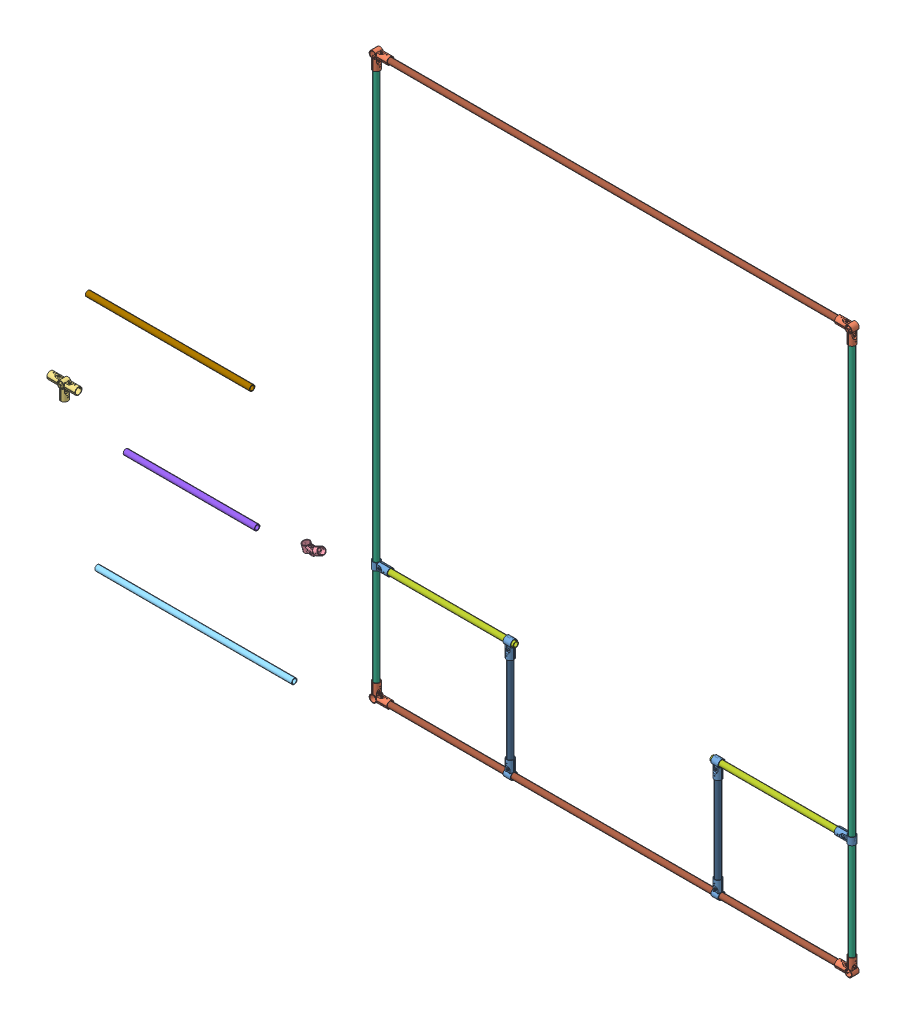
SolidWorks assembly SteelTubeAssembly, configuration Default. Lengths in mm.
Overall size (3905.99 2753.98 797.75).
23 component instances, 11 part files, 50 mates.
Components (placement in the parent):
- 2534T210_CLAMP-ON FRAMING FITTING-2: 2534T210_CLAMP-ON FRAMING FITTING [2534T21] at (584.2 0 0) x (1 0 0) z (0 0 -1) size (33.53 82.55 34.1)
- 2534T240_CLAMP-ON FRAMING FITTING-1: 2534T240_CLAMP-ON FRAMING FITTING [2534T24] at (2171.7 0 0) x (-1 0 0) z (0 0 1) size (81.85 81.28 33.46)
- 2534T260_CLAMP-ON FRAMING FITTING-1: 2534T260_CLAMP-ON FRAMING FITTING [2534T26] at (-1430.376 594.6399 57.1912) size (130.05 82.36 33.46)
- 2534T330_CLAMP-ON FRAMING FITTING-1: 2534T330_CLAMP-ON FRAMING FITTING [2534T33] at (46.223 849.693 406.2699) x (0.990082 0.041139 0.134332) z (-0.122317 -0.217936 0.968268) size (113.89 62.11 35.25)
- Depth Bar-1: Depth Bar [Default] at (-1338.4664 -133.7185 -4.7662) size (914.4 25.4 25.4)
- Height-1: Height [Default] at (2171.7 2552.7 0) x (0 -1 0) z (-0.85323 0 -0.521535) size (2514.6 25.4 25.4)
- Horizonal Corner-1: Horizonal Corner [Default] at (0 533.4 0) size (609.6 25.4 25.4)
- Lower Mounting Bar-1: Lower Mounting Bar [Default] at (-1489.6692 115.3649 -288.1125) size (609.6 25.4 25.4)
- Upper Mounting Bar-1: Upper Mounting Bar [Default] at (-1716.8304 613.4329 -339.6472) size (762 25.4 25.4)
- Vertical Corner-1: Vertical Corner [Default] at (584.2 495.3 0) x (0 -1 0) z (-0.899193 0 0.437553) size (457.2 25.4 25.4)
- Width-1: Width [Default] at origin size (2133.6 25.4 25.4)
- 2534T240_CLAMP-ON FRAMING FITTING-2: 2534T240_CLAMP-ON FRAMING FITTING [2534T24] at (2171.7 2590.8 0) x (-1 0 0) z (0 0 -1) size (81.85 81.28 33.46)
- 2534T240_CLAMP-ON FRAMING FITTING-5: 2534T240_CLAMP-ON FRAMING FITTING [2534T24] at (-38.1 0 0) x (1 0 0) z (0 0 -1) size (81.85 81.28 33.46)
- Height-3: Height [Default] at (-38.1 2552.7 0) x (0 -1 0) z (-0.845396 0 -0.534139) size (2514.6 25.4 25.4)
- 2534T240_CLAMP-ON FRAMING FITTING-6: 2534T240_CLAMP-ON FRAMING FITTING [2534T24] at (-38.1 2590.8 0) size (81.85 81.28 33.46)
- Width-3: Width [Default] at (0 2590.8 0) x (1 0 0) z (0 0.262637 0.964895) size (2133.6 25.4 25.4)
- 2534T210_CLAMP-ON FRAMING FITTING-3: 2534T210_CLAMP-ON FRAMING FITTING [2534T21] at (584.2 533.4 0) size (33.53 82.55 34.1)
- 2534T210_CLAMP-ON FRAMING FITTING-5: 2534T210_CLAMP-ON FRAMING FITTING [2534T21] at (-38.1 533.4 0) x (0 -1 0) z (0 0 -1) size (33.53 82.55 34.1)
- 2534T210_CLAMP-ON FRAMING FITTING-10: 2534T210_CLAMP-ON FRAMING FITTING [2534T21] at (1549.4 0 0) x (1 0 0) z (0 0 -1) size (33.53 82.55 34.1)
- 2534T210_CLAMP-ON FRAMING FITTING-11: 2534T210_CLAMP-ON FRAMING FITTING [2534T21] at (1549.4 533.4 0) x (-1 0 0) z (0 0 -1) size (33.53 82.55 34.1)
- Vertical Corner-3: Vertical Corner [Default] at (1549.4 495.3 0) x (0 -1 0) z (-0.962184 0 -0.272399) size (457.2 25.4 25.4)
- Horizonal Corner-3: Horizonal Corner [Default] at (1524 533.4 0) x (1 0 0) z (0 -0.195703 0.980663) size (609.6 25.4 25.4)
- 2534T210_CLAMP-ON FRAMING FITTING-12: 2534T210_CLAMP-ON FRAMING FITTING [2534T21] at (2171.7 533.4 0) x (0 -1 0) z (0 0 1) size (33.53 82.55 34.1)
Mates (geometry in assembly coordinates):
- Coincident1: coordinate: point of Width-1; point of assembly
- Concentric1: concentric anti-aligned: cylinder of 2534T240_CLAMP-ON FRAMING FITTING-1 through (2107.184 0 0) axis (1 0 0) radius 13.97; cylinder of Width-1 through (2133.6 0 0) axis (-1 0 0) radius 12.7
- Distance1: distance = 38.1 mm: point of 2534T240_CLAMP-ON FRAMING FITTING-1; plane of Width-1 through (2133.6 0 0) normal (1 0 0)
- Coincident2: coincident aligned: plane of Width-1 through (0 0 0) normal (0 0 1); plane of assembly through (0 0 0) normal (0 0 1)
- Parallel1: parallel aligned: plane of 2534T240_CLAMP-ON FRAMING FITTING-1 through (2171.7 64.516 0) normal (0 1 0); plane of assembly through (0 0 0) normal (0 1 0)
- Concentric2: concentric anti-aligned: cylinder of 2534T240_CLAMP-ON FRAMING FITTING-1 through (2171.7 64.516 0) axis (0 -1 0) radius 13.97; cylinder of Height-1 through (2171.7 38.1 0) axis (0 1 0) radius 12.7
- Distance2: distance = 38.1 mm anti-aligned: plane of Height-1 through (2171.7 38.1 0) normal (0 -1 0); plane of Width-1 through (0 0 0) normal (0 1 0)
- Concentric3: concentric aligned: cylinder of Height-1 through (2171.7 38.1 0) axis (0 1 0) radius 12.7; cylinder of 2534T240_CLAMP-ON FRAMING FITTING-2 through (2171.7 2526.284 0) axis (0 1 0) radius 13.97
- Distance3: distance = 38.1 mm: plane of Height-1 through (2171.7 2552.7 0) normal (0 1 0); point of 2534T240_CLAMP-ON FRAMING FITTING-2
- Parallel2: parallel aligned: plane of 2534T240_CLAMP-ON FRAMING FITTING-2 through (2171.7 2590.8 16.73) normal (0 0 1); plane of assembly through (0 0 0) normal (0 0 1)
- Concentric13: concentric aligned: cylinder of Width-1 through (2133.6 0 0) axis (-1 0 0) radius 12.7; cylinder of 2534T240_CLAMP-ON FRAMING FITTING-5 through (26.416 0 0) axis (-1 0 0) radius 13.97
- Distance9: distance = 38.1 mm: plane of Width-1 through (0 0 0) normal (-1 0 0); point of 2534T240_CLAMP-ON FRAMING FITTING-5
- Parallel5: parallel aligned: plane of 2534T240_CLAMP-ON FRAMING FITTING-1 through (2171.7 64.516 0) normal (0 1 0); plane of 2534T240_CLAMP-ON FRAMING FITTING-5 through (-38.1 64.516 0) normal (0 1 0)
- Concentric14: concentric anti-aligned: cylinder of 2534T240_CLAMP-ON FRAMING FITTING-5 through (-38.1 64.516 0) axis (0 -1 0) radius 13.97; cylinder of Height-3 through (-38.1 38.1 0) axis (0 1 0) radius 12.7
- Distance10: distance = 38.1 mm: plane of Height-3 through (-38.1 38.1 0) normal (0 -1 0); point of 2534T240_CLAMP-ON FRAMING FITTING-5
- Concentric15: concentric aligned: cylinder of Height-3 through (-38.1 38.1 0) axis (0 1 0) radius 12.7; cylinder of 2534T240_CLAMP-ON FRAMING FITTING-6 through (-38.1 2526.284 0) axis (0 1 0) radius 13.97
- Distance11: distance = 38.1 mm: plane of Height-3 through (-38.1 2552.7 0) normal (0 1 0); point of 2534T240_CLAMP-ON FRAMING FITTING-6
- Parallel6: parallel aligned: plane of Height-1 through (2171.7 2552.7 0) normal (0 1 0); plane of Height-3 through (-38.1 2552.7 0) normal (0 1 0)
- Concentric16: concentric anti-aligned: cylinder of 2534T240_CLAMP-ON FRAMING FITTING-2 through (2107.184 2590.8 0) axis (1 0 0) radius 13.97; cylinder of Width-3 through (2133.6 2590.8 0) axis (-1 0 0) radius 12.7
- Distance12: distance = 38.1 mm: point of 2534T240_CLAMP-ON FRAMING FITTING-2; plane of Width-3 through (2133.6 2590.8 0) normal (1 0 0)
- Parallel8: parallel anti-aligned: plane of 2534T240_CLAMP-ON FRAMING FITTING-2 through (2107.184 2590.8 0) normal (-1 0 0); plane of 2534T240_CLAMP-ON FRAMING FITTING-6 through (26.416 2590.8 0) normal (1 0 0)
- Concentric19: concentric aligned: cylinder of 2534T210_CLAMP-ON FRAMING FITTING-2 through (600.964 0 0) axis (-1 0 0) radius 13.97; cylinder of Width-1 through (2133.6 0 0) axis (-1 0 0) radius 12.7
- Parallel9: parallel aligned: plane of 2534T210_CLAMP-ON FRAMING FITTING-2 through (584.2 65.786 0) normal (0 1 0); plane of 2534T240_CLAMP-ON FRAMING FITTING-5 through (-38.1 64.516 0) normal (0 1 0)
- Concentric20: concentric anti-aligned: cylinder of 2534T210_CLAMP-ON FRAMING FITTING-2 through (584.2 65.786 0) axis (0 -1 0) radius 13.97; cylinder of Vertical Corner-1 through (584.2 38.1 0) axis (0 1 0) radius 12.7
- Distance13: distance = 38.1 mm: point of 2534T210_CLAMP-ON FRAMING FITTING-2; plane of Vertical Corner-1 through (584.2 38.1 0) normal (0 -1 0)
- Concentric24: concentric aligned: cylinder of Vertical Corner-1 through (584.2 38.1 0) axis (0 1 0) radius 12.7; cylinder of 2534T210_CLAMP-ON FRAMING FITTING-3 through (584.2 467.614 0) axis (0 1 0) radius 13.97
- Distance14: distance = 38.1 mm: point of 2534T210_CLAMP-ON FRAMING FITTING-3; plane of Vertical Corner-1 through (584.2 495.3 0) normal (0 1 0)
- Concentric25: concentric anti-aligned: cylinder of Height-3 through (-38.1 38.1 0) axis (0 1 0) radius 12.7; cylinder of 2534T210_CLAMP-ON FRAMING FITTING-5 through (-38.1 550.164 0) axis (0 -1 0) radius 13.97
- Parallel10: parallel aligned: plane of 2534T240_CLAMP-ON FRAMING FITTING-5 through (26.416 0 0) normal (1 0 0); plane of 2534T210_CLAMP-ON FRAMING FITTING-5 through (27.686 533.4 0) normal (1 0 0)
- Parallel11: parallel anti-aligned: plane of 2534T210_CLAMP-ON FRAMING FITTING-3 through (567.436 533.4 0) normal (-1 0 0); plane of 2534T210_CLAMP-ON FRAMING FITTING-5 through (27.686 533.4 0) normal (1 0 0)
- Concentric26: concentric aligned: cylinder of Horizonal Corner-1 through (609.6 533.4 0) axis (-1 0 0) radius 12.7; cylinder of 2534T210_CLAMP-ON FRAMING FITTING-3 through (600.964 533.4 0) axis (-1 0 0) radius 13.97
- Distance15: distance = 25.4 mm: point of 2534T210_CLAMP-ON FRAMING FITTING-3; plane of Horizonal Corner-1 through (609.6 533.4 0) normal (1 0 0)
- Distance16: distance = 38.1 mm: plane of Horizonal Corner-1 through (0 533.4 0) normal (-1 0 0); point of 2534T210_CLAMP-ON FRAMING FITTING-5
- Concentric27: concentric aligned: cylinder of Horizonal Corner-1 through (609.6 533.4 0) axis (-1 0 0) radius 12.7; cylinder of 2534T210_CLAMP-ON FRAMING FITTING-5 through (27.686 533.4 0) axis (-1 0 0) radius 13.97
- Concentric28: concentric aligned: cylinder of ? through (569.8292 2128.6091 5503.5233) axis (0 1 0) radius 12.7; cylinder of ? through (569.8292 2558.1231 5503.5233) axis (0 1 0) radius 13.97
- Distance17: distance = 25.4 mm: point of ?; plane of ? through (595.2292 2623.9091 5503.5233) normal (1 0 0)
- Distance19: distance = 38.1 mm: point of ?; plane of ? through (569.8292 2585.8091 5503.5233) normal (0 1 0)
- Concentric30: concentric aligned: cylinder of ? through (595.2292 2623.9091 5503.5233) axis (-1 0 0) radius 12.7; cylinder of ? through (586.5932 2623.9091 5503.5233) axis (-1 0 0) radius 13.97
- Concentric31: concentric anti-aligned: cylinder of Width-1 through (2133.6 0 0) axis (-1 0 0) radius 12.7; cylinder of 2534T210_CLAMP-ON FRAMING FITTING-10 through (1532.636 0 0) axis (1 0 0) radius 13.97
- Concentric32: concentric anti-aligned: cylinder of 2534T210_CLAMP-ON FRAMING FITTING-10 through (1549.4 65.786 0) axis (0 -1 0) radius 13.97; cylinder of Vertical Corner-3 through (1549.4 38.1 0) axis (0 1 0) radius 12.7
- Distance20: distance = 38.1 mm: plane of Vertical Corner-3 through (1549.4 38.1 0) normal (0 -1 0); point of 2534T210_CLAMP-ON FRAMING FITTING-10
- Concentric33: concentric aligned: cylinder of 2534T210_CLAMP-ON FRAMING FITTING-11 through (1549.4 467.614 0) axis (0 1 0) radius 13.97; cylinder of Vertical Corner-3 through (1549.4 38.1 0) axis (0 1 0) radius 12.7
- Parallel12: parallel aligned: plane of 2534T240_CLAMP-ON FRAMING FITTING-1 through (2171.7 64.516 0) normal (0 1 0); plane of Vertical Corner-3 through (1549.4 495.3 0) normal (0 1 0)
- Distance21: distance = 38.1 mm: point of 2534T210_CLAMP-ON FRAMING FITTING-11; plane of Vertical Corner-3 through (1549.4 495.3 0) normal (0 1 0)
- Parallel13: parallel anti-aligned: plane of 2534T210_CLAMP-ON FRAMING FITTING-3 through (600.964 533.4 0) normal (1 0 0); plane of 2534T210_CLAMP-ON FRAMING FITTING-11 through (1532.636 533.4 0) normal (-1 0 0)
- Concentric34: concentric aligned: cylinder of 2534T210_CLAMP-ON FRAMING FITTING-11 through (1566.164 533.4 0) axis (-1 0 0) radius 13.97; cylinder of Horizonal Corner-3 through (2133.6 533.4 0) axis (-1 0 0) radius 12.7
- Distance22: distance = 25.4 mm: point of 2534T210_CLAMP-ON FRAMING FITTING-11; plane of Horizonal Corner-3 through (1524 533.4 0) normal (-1 0 0)
- Concentric35: concentric anti-aligned: cylinder of Height-1 through (2171.7 38.1 0) axis (0 1 0) radius 12.7; cylinder of 2534T210_CLAMP-ON FRAMING FITTING-12 through (2171.7 550.164 0) axis (0 -1 0) radius 13.97
- Concentric36: concentric anti-aligned: cylinder of Horizonal Corner-3 through (2133.6 533.4 0) axis (-1 0 0) radius 12.7; cylinder of 2534T210_CLAMP-ON FRAMING FITTING-12 through (2105.914 533.4 0) axis (1 0 0) radius 13.97
- Distance23: distance = 38.1 mm: point of 2534T210_CLAMP-ON FRAMING FITTING-12; plane of Horizonal Corner-3 through (2133.6 533.4 0) normal (1 0 0)
